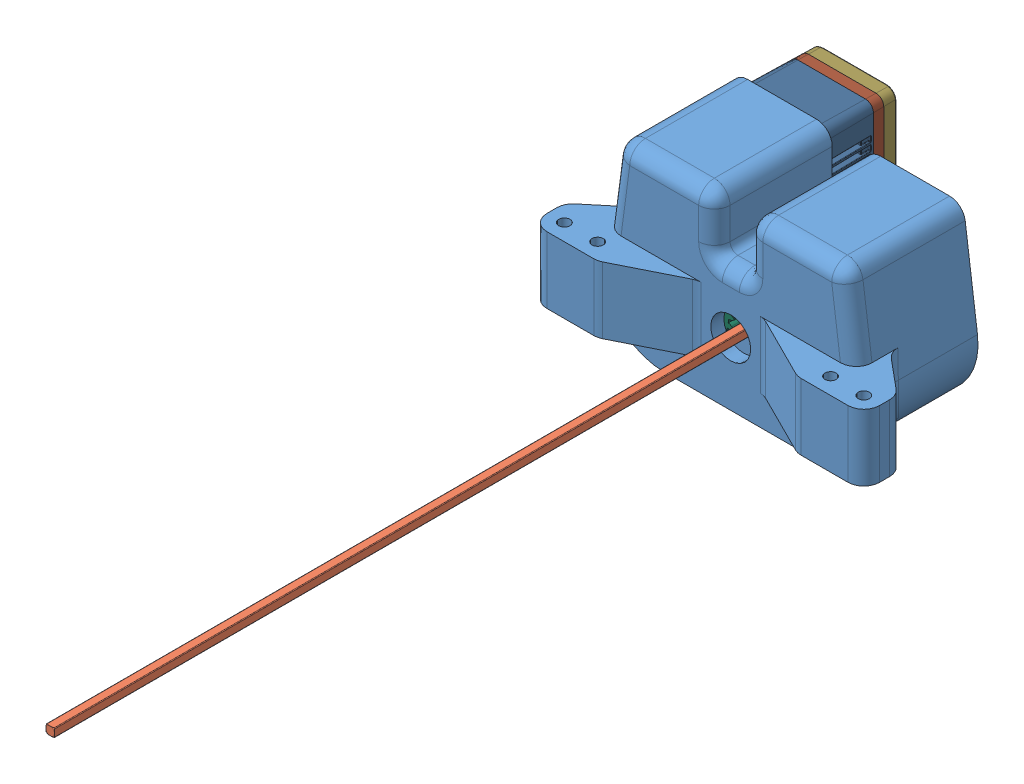
SolidWorks assembly Assem1, configuration Default. Lengths in mm.
Overall size (127 71.55 334.89).
24 component instances, 15 part files, 4 mates.
Components (placement in the parent):
- 2M_3to1_Gearbox-1: 2M_3to1_Gearbox [Default] at (41.3971 59.7632 105.3931) size (127 67.65 57.7)
- Drive Shaft 12_ (276-1149)-1: Drive Shaft 12_ (276-1149) [Default] at (41.4271 59.7483 217.7931) size (3.28 3.28 304.81)
- V5 Smart Motor (276-4840) no cap 3-1: V5 Smart Motor (276-4840) no cap 3 [Default] at (16.0633 72.4527 62.7121) x (0 -1 0) z (0 0 1) size (59.01 35.33 59.91)
  - V5 Smart Motor (276-4840).step-1: V5 Smart Motor (276-4840).step [Default] at origin size (59.01 35.33 59.91)
    - 276-4840-900 Rev6_Instruction.step-1: 276-4840-900 Rev6_Instruction.step [Default] at (-14.3 0 -17.2) size (52.79 15.94 38.15)
      - 276-4840-901 Rev6.step-1: 276-4840-901 Rev6.step [Default] at (10.75 -10.05 17.8) x (-1 0 0) z (0 0 1) size (49.9 1.6 38.15)
      - 276-4840-902 Rev2.step-1: 276-4840-902 Rev2.step [Default] at (31.25 -9.25 6.2) x (0 0 -1) z (0 -1 0) size (10.35 11.39 15.94)
      - 276-4840-022 Rev4.step-1: 276-4840-022 Rev4.step [Default] at (31.25 -9.25 6.2) x (0 0 -1) z (1 0 0) size (10.26 9.1 5.51)
    - 276-4840-110 Rev10_Instruction.step-1: 276-4840-110 Rev10_Instruction.step [Default] at (12.7 0 14.7) size (35.33 35.33 31.1)
      - 276-4840-061 Rev7_Ring_Gear_Fixed01 .6 Rev3.step-1: 276-4840-061 Rev7_Ring_Gear_Fixed01 .6 Rev3.step [Default] at origin size (28.79 28.39 24.6)
      - 276-4840-018 Rev6.step-1: 276-4840-018 Rev6.step [Default] at (0 0 6.7) x (-0.483174 0.875524 0) z (0 0 1) size (26 26 12.3)
      - 276-4840-059 Rev2.step-1: 276-4840-059 Rev2.step [Default] at (0 0 10.3) size (28.4 28.4 8.5)
      - 276-4840-062 Rev1.step-1: 276-4840-062 Rev1.step [Default] at (-12.1353 8.8168 12.3) x (0.956835 -0.290632 0) z (-0.290632 -0.956835 0) size (3.2 6.56 3.2)
      - 276-4840-062 Rev1.step-2: 276-4840-062 Rev1.step [Default] at (12.1353 8.8168 12.3) x (0.978427 0.206591 0) z (0.206591 -0.978427 0) size (3.2 6.56 3.2)
      - 276-4840-062 Rev1.step-3: 276-4840-062 Rev1.step [Default] at (-12.1353 -8.8168 12.3) x (0.72563 0.688086 0) z (0.688086 -0.72563 0) size (3.2 6.56 3.2)
    - 276-4840-001 Rev38.step-1: 276-4840-001 Rev38.step [Default] at origin size (57.3 33 46.9)
    - 276-4840-005 Rev27.step-1: 276-4840-005 Rev27.step [Default] at (0 0 -17.95) size (56.17 31.87 12.9)
    - 276-4840-004 Rev16.step-1: 276-4840-004 Rev16.step [Default] at (0 0 -19.2) size (56.01 31.71 9.21)
    - 276-4840-009 Rev3.step-1: 276-4840-009 Rev3.step [Default] at (25.45 13.5 15.7) x (0.19987 -0.979823 0) z (-0.979823 -0.19987 0) size (3.4 41.31 4.34)
    - 276-4840-009 Rev3.step-2: 276-4840-009 Rev3.step [Default] at (-25.45 -13.5 15.7) x (-0.998855 0.047836 0) z (0.047836 0.998855 0) size (3.4 41.31 4.34)
    - 276-4840-009 Rev3.step-3: 276-4840-009 Rev3.step [Default] at (25.45 -13.5 15.7) x (-0.975374 0.220559 0) z (0.220559 0.975374 0) size (3.4 41.31 4.34)
    - 276-4840-009 Rev3.step-4: 276-4840-009 Rev3.step [Default] at (-25.45 13.5 15.7) x (-0.922256 0.38658 0) z (0.38658 0.922256 0) size (3.4 41.31 4.34)
    - 276-4840-025 Rev19.step-1: 276-4840-025 Rev19.step [Default] at (12.7 0 -22.63) x (-0.993315 0.115437 0) z (0 0 1) size (14.82 14.83 35.18)
- 36T Gear (276-2169-002)-1: 36T Gear (276-2169-002) [Default] at (15.9971 59.7632 100.6306) x (-0.570584 -0.821239 0) z (0 0 1) size (40.08 40.08 9.53)
Mates (geometry in assembly coordinates):
- Coincident1: coincident aligned: plane of 2M_3to1_Gearbox-1 through (79.9471 97.4132 65.3931) normal (0 0 -1); plane of Drive Shaft 12_ (276-1149)-1 through (39.8396 61.3358 65.3931) normal (0 0 -1)
- Parallel1: parallel aligned: line of 2M_3to1_Gearbox-1 through (29.1471 101.0132 80.3931) axis (-1 0 0); line of V5 Smart Motor (276-4840) no cap 3-1/V5 Smart Motor (276-4840).step-1/276-4840-001 Rev38.step-1 through (28.9633 101.1027 78.9121) axis (-1 0 0)
- Concentric2: concentric anti-aligned: circle of 2M_3to1_Gearbox-1; circle of 36T Gear (276-2169-002)-1
- Coincident6: coincident anti-aligned: plane of 2M_3to1_Gearbox-1 through (41.3971 59.7632 105.3931) normal (0 0 -1); plane of 36T Gear (276-2169-002)-1 through (15.9971 59.7632 105.3931) normal (0 0 1)
